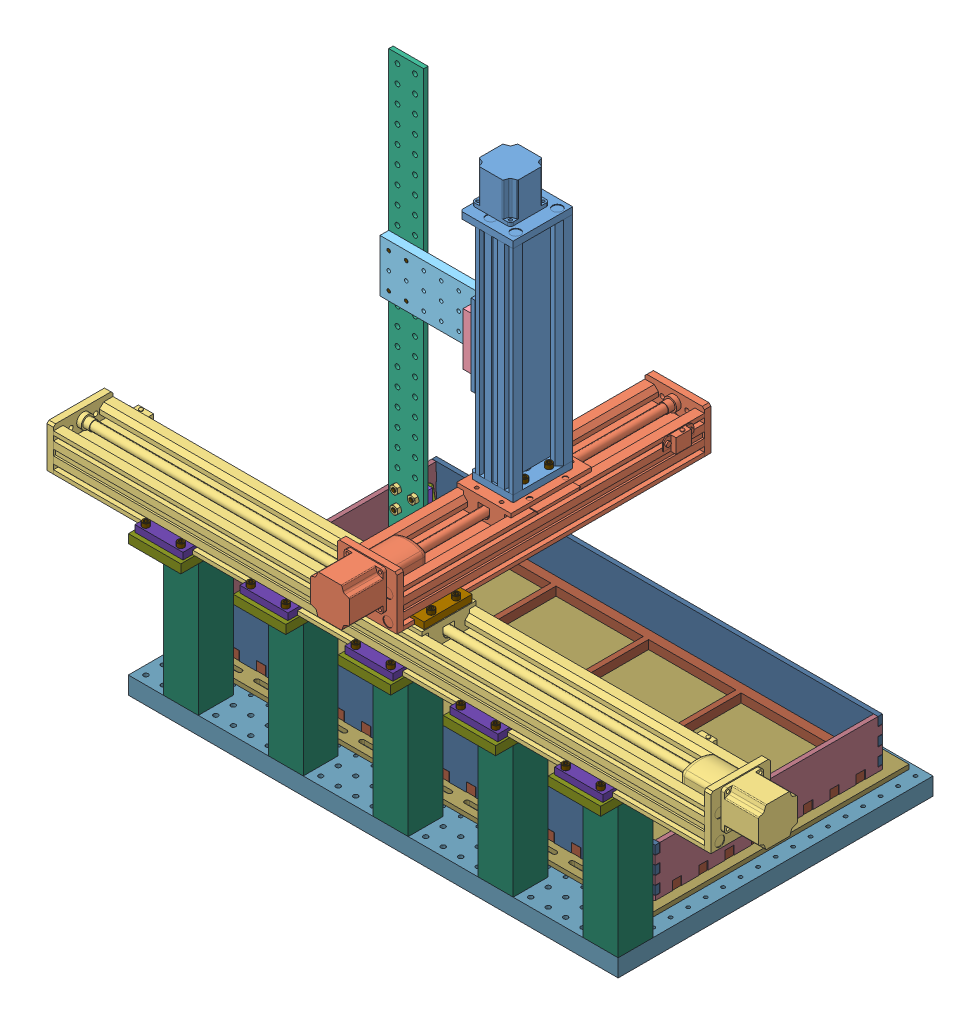
SolidWorks assembly Assem2, configuration Explosion. Lengths in mm.
Overall size (1018.03 802.77 546.22).
126 component instances, 21 part files, 120 mates.
Components (placement in the parent):
- MN10-0050-xxx-21 2Cleats PK266-1: MN10-0050-xxx-21 2Cleats PK266 [Default] at (26.0409 355.727 35.5482) x (0 0 -1) z (0 1 0) size (95.35 76.96 383.03)
- MN10-0100-xxx-21 2Cleats PK266-1: MN10-0100-xxx-21 2Cleats PK266 [Default] at (26.0409 308.3542 -182.8859) size (95.35 76.96 510.03)
- MN10-0300-xxx-21 2Cleats PK266-1: MN10-0300-xxx-21 2Cleats PK266 [Default] at (-446.405 243.2032 203.1941) x (0 0 -1) z (1 0 0) size (95.35 76.96 1018.03)
- Arm-1: Arm [Default] at (-11.8069 510.667 35.5482) x (0 0 1) z (0 -1 0) size (76.2 165.1 609.6)
  - Arm A-1: Arm A [Default] at origin size (76.2 12.7 76.2)
  - Arm B-1: Arm B [Default] at (0 88.9 0) x (0 1 0) z (0 0 1) size (152.4 12.7 76.2)
  - Arm C-1: Arm C [Default] at (-6.35 139.7 38.1) x (0 -1 0) z (0 0 -1) size (50.8 6.35 609.6)
- Verasonics (L11-5v)-1: Verasonics (L11-5v) [Default] at (-151.5069 115.5442 -3.8218) x (-1 0 0) z (0 0 1) size (57.98 122.43 23.49)
- L11_4v_holder_v8-1: L11_4v_holder_v8 [Default] at (-151.5069 155.067 -3.8218) size (50.8 114.3 26.72)
- BiSlide Cleat MC-2-1: BiSlide Cleat MC-2 [Default] at (69.2395 281.051 168.2691) size (20.27 9.74 69.85)
- BiSlide Cleat MC-2-2: BiSlide Cleat MC-2 [Default] at (-17.1695 281.051 238.1191) x (-1 0 0) z (0 0 -1) size (20.27 9.74 69.85)
- Tank-1: Tank [Default] at (-7.3117 0 -28.6003) size (674.12 76.2 382.02)
  - Tank_Long-1: Tank_Long [Default] at (0.508 47.625 -165.1) x (1 0 0) z (0 -1 0) size (647.7 6.35 75.69)
  - Tank_Inner-1: Tank_Inner [Default] at (0 6.35 0) size (647.7 12.7 330.2)
  - Tank_Base-1: Tank_Base [Default] at origin size (674.12 6.35 382.02)
  - Tank_Short-1: Tank_Short [Default] at (-323.342 47.625 0) x (0 0 -1) z (0 -1 0) size (330.2 6.35 75.69)
  - Tank_Short-2: Tank_Short [Default] at (318.008 47.625 -0.254) x (0 0 -1) z (0 -1 0) size (330.2 6.35 75.69)
  - Tank_Long-2: Tank_Long [Default] at (0.508 47.625 158.496) x (1 0 0) z (0 -1 0) size (647.7 6.35 75.69)
- Base-1: Base [Default] x (-1 0 0) z (0 0 -1) size (711.2 25.4 457.2)
- Pillar-5: Pillar [Default] at (330.2 0 203.2) size (50.8 203.2 50.8)
- Mount-1: Mount [Default] at (330.2 203.2 203.2) size (76.2 12.7 127)
- BiSlide Optical Table Cleat MC-3-1: BiSlide Optical Table Cleat MC-3 [Default] at (295.275 215.9 159.9955) x (0 0 -1) z (1 0 0) size (20.27 9.74 69.85)
- BiSlide Optical Table Cleat MC-3-2: BiSlide Optical Table Cleat MC-3 [Default] at (365.125 215.9 246.4045) x (0 0 1) z (-1 0 0) size (20.27 9.74 69.85)
- Screw 0.75-1: Screw 0.75 [92196A540] at (355.6 206.5945 152.4) x (0.967049 0 0.25459) z (0 -1 0) size (9.53 9.53 26.14)
- Screw 0.75-41: Screw 0.75 [92196A540] at (304.8 206.5945 152.4) x (0.928674 0 -0.370897) z (0 -1 0) size (9.53 9.53 26.14)
- Screw 0.75-46: Screw 0.75 [92196A540] at (304.8 206.5945 254) x (0.224681 0 -0.974432) z (0 -1 0) size (9.53 9.53 26.14)
- Screw 0.75-51: Screw 0.75 [92196A540] at (355.6 206.5945 254) x (0.019501 0 -0.99981) z (0 -1 0) size (9.53 9.53 26.14)
- Screw 1.00-2: Screw 1.00 [92196A542] at (317.5 8.89 215.9) x (1 0 0) z (0 1 0) size (9.53 9.53 32.53)
- Screw 1.00-22: Screw 1.00 [92196A542] at (342.9 8.89 215.9) x (1 0 0) z (0 1 0) size (9.53 9.53 32.53)
- Screw 1.00-27: Screw 1.00 [92196A542] at (317.5 8.89 190.5) x (1 0 0) z (0 1 0) size (9.53 9.53 32.53)
- Screw 1.00-32: Screw 1.00 [92196A542] at (342.9 8.89 190.5) x (1 0 0) z (0 1 0) size (9.53 9.53 32.53)
- Screw 0.75-56: Screw 0.75 [92196A540] at (342.9 190.5 215.9) x (0.019501 0 -0.99981) z (0 -1 0) size (9.53 9.53 26.14)
- Screw 0.75-61: Screw 0.75 [92196A540] at (342.9 190.5 190.5) x (0.019501 0 -0.99981) z (0 -1 0) size (9.53 9.53 26.14)
- Screw 0.75-66: Screw 0.75 [92196A540] at (317.5 190.5 215.9) x (0.019501 0 -0.99981) z (0 -1 0) size (9.53 9.53 26.14)
- Screw 0.75-71: Screw 0.75 [92196A540] at (317.5 190.5 190.5) x (0.320717 0 -0.947175) z (0 -1 0) size (9.53 9.53 26.14)
- Screw 0.75-72: Screw 0.75 [92196A540] at (165.1 190.5 190.5) x (0.320717 0 -0.947175) z (0 -1 0) size (9.53 9.53 26.14)
- Screw 0.75-73: Screw 0.75 [92196A540] at (12.7 190.5 190.5) x (0.320717 0 -0.947175) z (0 -1 0) size (9.53 9.53 26.14)
- Screw 0.75-74: Screw 0.75 [92196A540] at (-139.7 190.5 190.5) x (0.320717 0 -0.947175) z (0 -1 0) size (9.53 9.53 26.14)
- Screw 0.75-75: Screw 0.75 [92196A540] at (-292.1 190.5 190.5) x (0.320717 0 -0.947175) z (0 -1 0) size (9.53 9.53 26.14)
- Screw 0.75-67: Screw 0.75 [92196A540] at (165.1 190.5 215.9) x (0.019501 0 -0.99981) z (0 -1 0) size (9.53 9.53 26.14)
- Screw 0.75-68: Screw 0.75 [92196A540] at (12.7 190.5 215.9) x (0.019501 0 -0.99981) z (0 -1 0) size (9.53 9.53 26.14)
- Screw 0.75-69: Screw 0.75 [92196A540] at (-139.7 190.5 215.9) x (0.019501 0 -0.99981) z (0 -1 0) size (9.53 9.53 26.14)
- Screw 0.75-70: Screw 0.75 [92196A540] at (-292.1 190.5 215.9) x (0.019501 0 -0.99981) z (0 -1 0) size (9.53 9.53 26.14)
- Screw 0.75-62: Screw 0.75 [92196A540] at (190.5 190.5 190.5) x (0.019501 0 -0.99981) z (0 -1 0) size (9.53 9.53 26.14)
- Screw 0.75-63: Screw 0.75 [92196A540] at (38.1 190.5 190.5) x (0.019501 0 -0.99981) z (0 -1 0) size (9.53 9.53 26.14)
- Screw 0.75-64: Screw 0.75 [92196A540] at (-114.3 190.5 190.5) x (0.019501 0 -0.99981) z (0 -1 0) size (9.53 9.53 26.14)
- Screw 0.75-65: Screw 0.75 [92196A540] at (-266.7 190.5 190.5) x (0.019501 0 -0.99981) z (0 -1 0) size (9.53 9.53 26.14)
- Screw 0.75-57: Screw 0.75 [92196A540] at (190.5 190.5 215.9) x (0.019501 0 -0.99981) z (0 -1 0) size (9.53 9.53 26.14)
- Screw 0.75-58: Screw 0.75 [92196A540] at (38.1 190.5 215.9) x (0.019501 0 -0.99981) z (0 -1 0) size (9.53 9.53 26.14)
- Screw 0.75-59: Screw 0.75 [92196A540] at (-114.3 190.5 215.9) x (0.019501 0 -0.99981) z (0 -1 0) size (9.53 9.53 26.14)
- Screw 0.75-60: Screw 0.75 [92196A540] at (-266.7 190.5 215.9) x (0.019501 0 -0.99981) z (0 -1 0) size (9.53 9.53 26.14)
- Screw 1.00-33: Screw 1.00 [92196A542] at (190.5 8.89 190.5) x (1 0 0) z (0 1 0) size (9.53 9.53 32.53)
- Screw 1.00-34: Screw 1.00 [92196A542] at (38.1 8.89 190.5) x (1 0 0) z (0 1 0) size (9.53 9.53 32.53)
- Screw 1.00-35: Screw 1.00 [92196A542] at (-114.3 8.89 190.5) x (1 0 0) z (0 1 0) size (9.53 9.53 32.53)
- Screw 1.00-36: Screw 1.00 [92196A542] at (-266.7 8.89 190.5) x (1 0 0) z (0 1 0) size (9.53 9.53 32.53)
- Screw 1.00-28: Screw 1.00 [92196A542] at (165.1 8.89 190.5) x (1 0 0) z (0 1 0) size (9.53 9.53 32.53)
- Screw 1.00-29: Screw 1.00 [92196A542] at (12.7 8.89 190.5) x (1 0 0) z (0 1 0) size (9.53 9.53 32.53)
- Screw 1.00-30: Screw 1.00 [92196A542] at (-139.7 8.89 190.5) x (1 0 0) z (0 1 0) size (9.53 9.53 32.53)
- Screw 1.00-31: Screw 1.00 [92196A542] at (-292.1 8.89 190.5) x (1 0 0) z (0 1 0) size (9.53 9.53 32.53)
- Screw 1.00-23: Screw 1.00 [92196A542] at (190.5 8.89 215.9) x (1 0 0) z (0 1 0) size (9.53 9.53 32.53)
- Screw 1.00-24: Screw 1.00 [92196A542] at (38.1 8.89 215.9) x (1 0 0) z (0 1 0) size (9.53 9.53 32.53)
- Screw 1.00-25: Screw 1.00 [92196A542] at (-114.3 8.89 215.9) x (1 0 0) z (0 1 0) size (9.53 9.53 32.53)
- Screw 1.00-26: Screw 1.00 [92196A542] at (-266.7 8.89 215.9) x (1 0 0) z (0 1 0) size (9.53 9.53 32.53)
- Screw 1.00-18: Screw 1.00 [92196A542] at (165.1 8.89 215.9) x (1 0 0) z (0 1 0) size (9.53 9.53 32.53)
- Screw 1.00-19: Screw 1.00 [92196A542] at (12.7 8.89 215.9) x (1 0 0) z (0 1 0) size (9.53 9.53 32.53)
- Screw 1.00-20: Screw 1.00 [92196A542] at (-139.7 8.89 215.9) x (1 0 0) z (0 1 0) size (9.53 9.53 32.53)
- Screw 1.00-21: Screw 1.00 [92196A542] at (-292.1 8.89 215.9) x (1 0 0) z (0 1 0) size (9.53 9.53 32.53)
- Screw 0.75-52: Screw 0.75 [92196A540] at (203.2 206.5945 254) x (0.019501 0 -0.99981) z (0 -1 0) size (9.53 9.53 26.14)
- Screw 0.75-53: Screw 0.75 [92196A540] at (50.8 206.5945 254) x (0.019501 0 -0.99981) z (0 -1 0) size (9.53 9.53 26.14)
- Screw 0.75-54: Screw 0.75 [92196A540] at (-101.6 206.5945 254) x (0.019501 0 -0.99981) z (0 -1 0) size (9.53 9.53 26.14)
- Screw 0.75-55: Screw 0.75 [92196A540] at (-254 206.5945 254) x (0.019501 0 -0.99981) z (0 -1 0) size (9.53 9.53 26.14)
- Screw 0.75-47: Screw 0.75 [92196A540] at (152.4 206.5945 254) x (0.224681 0 -0.974432) z (0 -1 0) size (9.53 9.53 26.14)
- Screw 0.75-48: Screw 0.75 [92196A540] at (0 206.5945 254) x (0.224681 0 -0.974432) z (0 -1 0) size (9.53 9.53 26.14)
- Screw 0.75-49: Screw 0.75 [92196A540] at (-152.4 206.5945 254) x (0.224681 0 -0.974432) z (0 -1 0) size (9.53 9.53 26.14)
- Screw 0.75-50: Screw 0.75 [92196A540] at (-304.8 206.5945 254) x (0.224681 0 -0.974432) z (0 -1 0) size (9.53 9.53 26.14)
- Screw 0.75-42: Screw 0.75 [92196A540] at (152.4 206.5945 152.4) x (0.928674 0 -0.370897) z (0 -1 0) size (9.53 9.53 26.14)
- Screw 0.75-43: Screw 0.75 [92196A540] at (0 206.5945 152.4) x (0.928674 0 -0.370897) z (0 -1 0) size (9.53 9.53 26.14)
- Screw 0.75-44: Screw 0.75 [92196A540] at (-152.4 206.5945 152.4) x (0.928674 0 -0.370897) z (0 -1 0) size (9.53 9.53 26.14)
- Screw 0.75-45: Screw 0.75 [92196A540] at (-304.8 206.5945 152.4) x (0.928674 0 -0.370897) z (0 -1 0) size (9.53 9.53 26.14)
- Screw 0.75-37: Screw 0.75 [92196A540] at (203.2 206.5945 152.4) x (0.967049 0 0.25459) z (0 -1 0) size (9.53 9.53 26.14)
- Screw 0.75-38: Screw 0.75 [92196A540] at (50.8 206.5945 152.4) x (0.967049 0 0.25459) z (0 -1 0) size (9.53 9.53 26.14)
- Screw 0.75-39: Screw 0.75 [92196A540] at (-101.6 206.5945 152.4) x (0.967049 0 0.25459) z (0 -1 0) size (9.53 9.53 26.14)
- Screw 0.75-40: Screw 0.75 [92196A540] at (-254 206.5945 152.4) x (0.967049 0 0.25459) z (0 -1 0) size (9.53 9.53 26.14)
- BiSlide Optical Table Cleat MC-3-11: BiSlide Optical Table Cleat MC-3 [Default] at (212.725 215.9 246.4045) x (0 0 1) z (-1 0 0) size (20.27 9.74 69.85)
- BiSlide Optical Table Cleat MC-3-12: BiSlide Optical Table Cleat MC-3 [Default] at (60.325 215.9 246.4045) x (0 0 1) z (-1 0 0) size (20.27 9.74 69.85)
- BiSlide Optical Table Cleat MC-3-13: BiSlide Optical Table Cleat MC-3 [Default] at (-92.075 215.9 246.4045) x (0 0 1) z (-1 0 0) size (20.27 9.74 69.85)
- BiSlide Optical Table Cleat MC-3-14: BiSlide Optical Table Cleat MC-3 [Default] at (-244.475 215.9 246.4045) x (0 0 1) z (-1 0 0) size (20.27 9.74 69.85)
- BiSlide Optical Table Cleat MC-3-15: BiSlide Optical Table Cleat MC-3 [Default] at (142.875 215.9 159.9955) x (0 0 -1) z (1 0 0) size (20.27 9.74 69.85)
- BiSlide Optical Table Cleat MC-3-16: BiSlide Optical Table Cleat MC-3 [Default] at (-9.525 215.9 159.9955) x (0 0 -1) z (1 0 0) size (20.27 9.74 69.85)
- BiSlide Optical Table Cleat MC-3-17: BiSlide Optical Table Cleat MC-3 [Default] at (-161.925 215.9 159.9955) x (0 0 -1) z (1 0 0) size (20.27 9.74 69.85)
- BiSlide Optical Table Cleat MC-3-18: BiSlide Optical Table Cleat MC-3 [Default] at (-314.325 215.9 159.9955) x (0 0 -1) z (1 0 0) size (20.27 9.74 69.85)
- Mount-6: Mount [Default] at (177.8 203.2 203.2) size (76.2 12.7 127)
- Mount-7: Mount [Default] at (25.4 203.2 203.2) size (76.2 12.7 127)
- Mount-8: Mount [Default] at (-127 203.2 203.2) size (76.2 12.7 127)
- Mount-9: Mount [Default] at (-279.4 203.2 203.2) size (76.2 12.7 127)
- Pillar-10: Pillar [Default] at (177.8 0 203.2) size (50.8 203.2 50.8)
- Pillar-11: Pillar [Default] at (25.4 0 203.2) size (50.8 203.2 50.8)
- Pillar-12: Pillar [Default] at (-127 0 203.2) size (50.8 203.2 50.8)
- Pillar-13: Pillar [Default] at (-279.4 0 203.2) size (50.8 203.2 50.8)
- Screw 0.75-76: Screw 0.75 [92196A540] at (76.835 271.7455 185.1601) x (0.380553 0 0.924759) z (0 -1 0) size (9.53 9.53 26.14)
- Screw 0.75-77: Screw 0.75 [92196A540] at (76.835 271.7455 221.2281) x (0.931591 0 0.363508) z (0 -1 0) size (9.53 9.53 26.14)
- Screw 0.75-78: Screw 0.75 [92196A540] at (-24.765 271.7455 185.1601) x (-0.20973 0 -0.977759) z (0 -1 0) size (9.53 9.53 26.14)
- Screw 0.75-79: Screw 0.75 [92196A540] at (-24.765 271.7455 221.2281) x (0.199431 0 -0.979912) z (0 -1 0) size (9.53 9.53 26.14)
- Screw 0.75-80: Screw 0.75 [92196A540] at (44.0749 336.677 53.5881) x (0.844393 0 0.535724) z (0 -1 0) size (9.53 9.53 26.14)
- Screw 0.75-81: Screw 0.75 [92196A540] at (44.0749 336.677 17.5201) x (0.224867 0 -0.974389) z (0 -1 0) size (9.53 9.53 26.14)
- Screw 0.75-82: Screw 0.75 [92196A540] at (8.0069 336.677 17.5201) x (-0.995611 0 -0.093586) z (0 -1 0) size (9.53 9.53 26.14)
- Screw 0.75-83: Screw 0.75 [92196A540] at (8.0069 336.677 53.5881) x (-0.995611 0 -0.093586) z (0 -1 0) size (9.53 9.53 26.14)
- Screw 0.50-1: Screw 0.50 [92196A537] at (-5.4569 528.701 53.5822) x (0 0.678478 -0.734621) z (1 0 0) size (9.53 9.53 19.76)
- Screw 0.50-2: Screw 0.50 [92196A537] at (-5.4569 492.633 53.5822) x (0 0.678478 -0.734621) z (1 0 0) size (9.53 9.53 19.76)
- Screw 0.50-4: Screw 0.50 [92196A537] at (-5.4569 492.633 17.5142) x (0 0.678478 -0.734621) z (1 0 0) size (9.53 9.53 19.76)
- Screw 0.50-5: Screw 0.50 [92196A537] at (-5.4569 528.701 17.5142) x (0 0.84628 0.532739) z (1 0 0) size (9.53 9.53 19.76)
- Screw 0.50-6: Screw 0.50 [92196A537] at (-30.8569 485.267 35.5482) x (0 -0.902178 -0.431364) z (-1 0 0) size (9.53 9.53 19.76)
- Screw 0.50-7: Screw 0.50 [92196A537] at (-30.8569 510.667 35.5482) x (0 0.454026 -0.890989) z (-1 0 0) size (9.53 9.53 19.76)
- Screw 0.50-8: Screw 0.50 [92196A537] at (-30.8569 536.067 35.5482) x (0 0.397067 -0.91779) z (-1 0 0) size (9.53 9.53 19.76)
- Screw 0.75-84: Screw 0.75 [92196A540] at (-138.8069 536.067 41.8982) x (0.718354 -0.695678 0) z (0 0 1) size (9.53 9.53 26.14)
- Screw 0.75-85: Screw 0.75 [92196A540] at (-164.2069 536.067 41.8982) x (-0.621869 -0.783122 0) z (0 0 1) size (9.53 9.53 26.14)
- Screw 0.75-86: Screw 0.75 [92196A540] at (-138.8069 485.267 41.8982) x (-0.621869 -0.783122 0) z (0 0 1) size (9.53 9.53 26.14)
- Screw 0.75-87: Screw 0.75 [92196A540] at (-164.2069 485.267 41.8982) x (-0.621869 -0.783122 0) z (0 0 1) size (9.53 9.53 26.14)
- Screw 0.75-88: Screw 0.75 [92196A540] at (-164.2069 205.867 35.5482) x (-0.621869 -0.783122 0) z (0 0 1) size (9.53 9.53 26.14)
- Screw 0.75-89: Screw 0.75 [92196A540] at (-138.8069 231.267 35.5482) x (-0.621869 -0.783122 0) z (0 0 1) size (9.53 9.53 26.14)
- Screw 0.75-90: Screw 0.75 [92196A540] at (-138.8069 205.867 35.5482) x (-0.621869 -0.783122 0) z (0 0 1) size (9.53 9.53 26.14)
- Screw 0.75-91: Screw 0.75 [92196A540] at (-164.2069 231.267 35.5482) x (-0.621869 -0.783122 0) z (0 0 1) size (9.53 9.53 26.14)
- Nut-1: Nut [91845A029] at (-164.2069 231.267 31.9763) x (0.978932 0.204188 0) z (0 0 1) size (11.11 12.83 6.51)
- Nut-2: Nut [91845A029] at (-138.8069 231.267 31.9763) x (0.978932 0.204188 0) z (0 0 1) size (11.11 12.83 6.51)
- Nut-3: Nut [91845A029] at (-164.2069 205.867 31.9763) x (0.978932 0.204188 0) z (0 0 1) size (11.11 12.83 6.51)
- Nut-4: Nut [91845A029] at (-138.8069 205.867 31.9763) x (0.978932 0.204188 0) z (0 0 1) size (11.11 12.83 6.51)
Mates (geometry in assembly coordinates):
- Coincident64: coincident anti-aligned: plane of MN10-0300-xxx-21 2Cleats PK266-1 through (-446.405 221.6132 159.9946) normal (0 0 -1); plane of BiSlide Optical Table Cleat MC-3-1 through (295.275 218.7566 159.9946) normal (0 0 1)
- Coincident65: coincident anti-aligned: plane of MN10-0300-xxx-21 2Cleats PK266-1 through (-446.405 221.6132 166.7583) normal (0 1 0); plane of BiSlide Optical Table Cleat MC-3-1 through (295.275 221.6132 163.1569) normal (0 -1 0)
- Coincident66: coincident anti-aligned: plane of Pillar-5 through (330.2 203.2 203.2) normal (0 1 0); plane of Mount-1 through (330.2 203.2 203.2) normal (0 -1 0)
- Parallel1: parallel aligned: plane of Pillar-5 through (304.8 203.2 177.8) normal (0 0 -1); plane of Mount-1 through (292.1 215.9 139.7) normal (0 0 -1)
- Coincident67: coincident anti-aligned: plane of MN10-0300-xxx-21 2Cleats PK266-1 through (-446.405 215.9 246.4054) normal (0 0 1); plane of BiSlide Optical Table Cleat MC-3-2 through (365.125 218.7566 246.4054) normal (0 0 -1)
- Coincident68: coincident anti-aligned: plane of MN10-0300-xxx-21 2Cleats PK266-1 through (-446.405 221.6132 246.4054) normal (0 1 0); plane of BiSlide Optical Table Cleat MC-3-2 through (365.125 221.6132 243.2431) normal (0 -1 0)
- Coincident69: coincident anti-aligned: plane of MN10-0300-xxx-21 2Cleats PK266-1 through (-446.405 215.9 232.7392) normal (0 -1 0); plane of Mount-1 through (330.2 215.9 203.2) normal (0 1 0)
- Coincident70: coincident anti-aligned: plane of MN10-0300-xxx-21 2Cleats PK266-1 through (-32.385 281.051 242.5439) normal (0 1 0); plane of MN10-0100-xxx-21 2Cleats PK266-1 through (69.2404 281.051 253.9941) normal (0 -1 0)
- Parallel2: parallel anti-aligned: line of MN10-0300-xxx-21 2Cleats PK266-1 through (84.455 275.3631 242.5439) axis (0 1 0); line of MN10-0100-xxx-21 2Cleats PK266-1 through (69.2404 355.0614 263.5191) axis (0 -1 0)
- Coincident74: coincident anti-aligned: plane of MN10-0100-xxx-21 2Cleats PK266-1 through (-13.3089 346.202 -22.8659) normal (0 1 0); plane of MN10-0050-xxx-21 2Cleats PK266-1 through (22.7334 346.202 35.5546) normal (0 -1 0)
- Parallel3: parallel aligned: plane of MN10-0100-xxx-21 2Cleats PK266-1 through (26.0347 328.2952 317.6211) normal (0 0 1); plane of MN10-0050-xxx-21 2Cleats PK266-1 through (21.8502 355.727 78.7595) normal (0 0 1)
- Coincident75: coincident anti-aligned: plane of Base-1 through (0 0 0) normal (0 1 0); plane of Tank-1/Tank_Base-1 through (-7.3117 0 -28.6003) normal (0 -1 0)
- Concentric35: concentric anti-aligned: circle of L11_4v_holder_v8-1; circle of Verasonics (L11-5v)-1
- Parallel8: parallel aligned: plane of L11_4v_holder_v8-1 through (-176.9069 104.267 10.1482) normal (-1 0 0); plane of Verasonics (L11-5v)-1 through (-151.5069 115.5442 -3.8218) normal (-1 0 0)
- Distance2: distance = 44.0772 mm aligned: plane of Verasonics (L11-5v)-1 through (-151.5069 224.5442 -3.8218) normal (0 1 0); plane of L11_4v_holder_v8-1 through (-151.5069 180.467 -3.8218) normal (0 1 0)
- Parallel9: parallel aligned: plane of MN10-0050-xxx-21 2Cleats PK266-1 through (1.2787 569.087 35.5482) normal (0 1 0); plane of Arm-1/Arm B-1 through (-24.5069 548.767 29.1982) normal (0 1 0)
- Parallel10: parallel aligned: plane of Arm-1/Arm C-1 through (-176.9069 777.367 22.8482) normal (-1 0 0); plane of L11_4v_holder_v8-1 through (-176.9069 104.267 10.1482) normal (-1 0 0)
- Concentric38: concentric aligned: circle of Arm-1/Arm C-1; circle of L11_4v_holder_v8-1
- Concentric39: concentric aligned: circle of Arm-1/Arm C-1; circle of L11_4v_holder_v8-1
- Coincident81: coincident anti-aligned: plane of Arm-1/Arm C-1 through (-151.5069 472.567 22.8482) normal (0 0 -1); plane of L11_4v_holder_v8-1 through (-151.5069 155.067 22.8482) normal (0 0 1)
- Coincident82: coincident anti-aligned: plane of MN10-0050-xxx-21 2Cleats PK266-1 through (-11.8069 452.247 74.898) normal (-1 0 0); plane of Arm-1/Arm A-1 through (-11.8069 510.667 35.5482) normal (1 0 0)
- Concentric41: concentric anti-aligned: circle of MN10-0050-xxx-21 2Cleats PK266-1; circle of Arm-1/Arm A-1
- Coincident83: coincident anti-aligned: plane of MN10-0300-xxx-21 2Cleats PK266-1 through (-32.385 281.051 242.5439) normal (0 1 0); plane of BiSlide Cleat MC-2-1 through (83.185 281.051 168.2691) normal (0 -1 0)
- Concentric42: concentric aligned: circle of MN10-0300-xxx-21 2Cleats PK266-1; circle of BiSlide Cleat MC-2-1
- Parallel11: parallel aligned: plane of MN10-0300-xxx-21 2Cleats PK266-1 through (84.455 267.9653 203.1941) normal (1 0 0); plane of BiSlide Cleat MC-2-1 through (83.185 290.7955 168.2691) normal (1 0 0)
- Distance3: distance = 25.4 mm aligned: plane of MN10-0100-xxx-21 2Cleats PK266-1 through (26.0345 319.1099 263.5191) normal (0 0 1); plane of BiSlide Cleat MC-2-1 through (73.6524 286.5252 238.1191) normal (0 0 1)
- Concentric43: concentric anti-aligned: circle of MN10-0300-xxx-21 2Cleats PK266-1; cylinder of BiSlide Cleat MC-2-2 through (-24.765 217.4142 185.1601) axis (0 1 0) radius 3.4544
- Parallel12: parallel aligned: plane of MN10-0300-xxx-21 2Cleats PK266-1 through (-32.385 267.9653 203.1941) normal (-1 0 0); plane of BiSlide Cleat MC-2-2 through (-31.115 290.7955 238.1191) normal (-1 0 0)
- Coincident84: coincident anti-aligned: plane of MN10-0300-xxx-21 2Cleats PK266-1 through (-32.385 281.051 242.5439) normal (0 1 0); plane of BiSlide Cleat MC-2-2 through (-31.115 281.051 238.1191) normal (0 -1 0)
- Concentric47: concentric aligned: circle of BiSlide Optical Table Cleat MC-3-1; cylinder of Screw 0.75-1 through (355.6 231.9945 152.4) axis (0 -1 0) radius 4.7625
- Concentric48: concentric aligned: cylinder of BiSlide Optical Table Cleat MC-3-1 through (355.6 152.2632 152.4) axis (0 1 0) radius 3.4544; cylinder of Mount-1 through (355.6 215.9 152.4) axis (0 1 0) radius 2.5527
- Coincident87: coincident anti-aligned: plane of BiSlide Optical Table Cleat MC-3-1 through (295.275 225.6445 156.1846) normal (0 1 0); plane of Screw 0.75-1 through (355.6 225.6445 152.4) normal (0 -1 0)
- Coincident88: coincident anti-aligned: plane of BiSlide Optical Table Cleat MC-3-1 through (295.275 225.6445 156.1846) normal (0 1 0); plane of Screw 0.75-41 through (304.8 225.6445 152.4) normal (0 -1 0)
- Concentric49: concentric anti-aligned: cylinder of BiSlide Optical Table Cleat MC-3-1 through (304.8 152.2632 152.4) axis (0 1 0) radius 3.4544; cylinder of Screw 0.75-41 through (304.8 231.9945 152.4) axis (0 -1 0) radius 4.7625
- Concentric50: concentric aligned: cylinder of BiSlide Optical Table Cleat MC-3-2 through (304.8 152.2632 254) axis (0 1 0) radius 3.4544; cylinder of Mount-1 through (304.8 215.9 254) axis (0 1 0) radius 2.5527
- Concentric51: concentric anti-aligned: cylinder of BiSlide Optical Table Cleat MC-3-2 through (355.6 152.2632 254) axis (0 1 0) radius 3.4544; cylinder of Screw 0.75-51 through (355.6 231.9945 254) axis (0 -1 0) radius 4.7625
- Concentric52: concentric anti-aligned: cylinder of BiSlide Optical Table Cleat MC-3-2 through (304.8 152.2632 254) axis (0 1 0) radius 3.4544; cylinder of Screw 0.75-46 through (304.8 231.9945 254) axis (0 -1 0) radius 4.7625
- Coincident89: coincident aligned: plane of Screw 0.75-1 through (355.6 231.9945 152.4) normal (0 1 0); plane of Screw 0.75-51 through (355.6 231.9945 254) normal (0 1 0)
- Coincident90: coincident aligned: plane of Screw 0.75-46 through (304.8 231.9945 254) normal (0 1 0); plane of Screw 0.75-51 through (355.6 231.9945 254) normal (0 1 0)
- Coincident91: coincident aligned: plane of Base-1 through (0 0 0) normal (0 1 0); plane of assembly through (0 0 0) normal (0 1 0)
- Coincident92: coincident anti-aligned: plane of Base-1 through (0 0 0) normal (-1 0 0); plane of assembly through (0 0 0) normal (1 0 0)
- Coincident93: coincident anti-aligned: plane of Base-1 through (0 0 0) normal (0 0 -1); plane of assembly through (0 0 0) normal (0 0 1)
- Coincident94: coincident anti-aligned: plane of Base-1 through (288.7218 -16.51 215.9) normal (0 -1 0); plane of Screw 1.00-2 through (317.5 -16.51 215.9) normal (0 1 0)
- Concentric54: concentric anti-aligned: cylinder of Base-1 through (317.5 -25.4 215.9) axis (0 -1 0) radius 5.5563; cylinder of Screw 1.00-2 through (317.5 -22.86 215.9) axis (0 1 0) radius 4.7625
- Concentric56: concentric anti-aligned: cylinder of Base-1 through (342.9 -25.4 215.9) axis (0 -1 0) radius 5.5563; cylinder of Screw 1.00-22 through (342.9 -22.86 215.9) axis (0 1 0) radius 4.7625
- Concentric57: concentric anti-aligned: cylinder of Base-1 through (317.5 -25.4 190.5) axis (0 -1 0) radius 5.5563; cylinder of Screw 1.00-27 through (317.5 -22.86 190.5) axis (0 1 0) radius 4.7625
- Concentric58: concentric anti-aligned: cylinder of Base-1 through (342.9 -25.4 190.5) axis (0 -1 0) radius 5.5563; cylinder of Screw 1.00-32 through (342.9 -22.86 190.5) axis (0 1 0) radius 4.7625
- Coincident96: coincident aligned: plane of Screw 1.00-2 through (319.8813 -19.2881 211.7756) normal (0 -1 0); plane of Screw 1.00-32 through (345.2812 -19.2881 186.3756) normal (0 -1 0)
- Coincident97: coincident aligned: plane of Screw 1.00-22 through (345.2812 -19.2881 211.7756) normal (0 -1 0); plane of Screw 1.00-32 through (345.2812 -19.2881 186.3756) normal (0 -1 0)
- Coincident98: coincident aligned: plane of Screw 1.00-27 through (319.8813 -19.2881 186.3756) normal (0 -1 0); plane of Screw 1.00-32 through (345.2812 -19.2881 186.3756) normal (0 -1 0)
- Coincident99: coincident anti-aligned: plane of Pillar-5 through (330.2 0 203.2) normal (0 -1 0); plane of Base-1 through (0 0 0) normal (0 1 0)
- Concentric61: concentric anti-aligned: cylinder of Mount-1 through (342.9 215.9 215.9) axis (0 1 0) radius 5.5563; cylinder of Screw 0.75-56 through (342.9 215.9 215.9) axis (0 -1 0) radius 4.7625
- Concentric62: concentric anti-aligned: cylinder of Mount-1 through (317.5 215.9 215.9) axis (0 1 0) radius 5.5563; cylinder of Screw 0.75-66 through (317.5 215.9 215.9) axis (0 -1 0) radius 4.7625
- Concentric63: concentric anti-aligned: cylinder of Mount-1 through (342.9 215.9 190.5) axis (0 1 0) radius 5.5563; cylinder of Screw 0.75-61 through (342.9 215.9 190.5) axis (0 -1 0) radius 4.7625
- Concentric64: concentric anti-aligned: cylinder of Mount-1 through (317.5 215.9 190.5) axis (0 1 0) radius 5.5563; cylinder of Screw 0.75-71 through (317.5 215.9 190.5) axis (0 -1 0) radius 4.7625
- Parallel13: parallel aligned: plane of Pillar-5 through (355.6 203.2 228.6) normal (1 0 0); plane of Base-1 through (355.6 -25.4 -228.6) normal (1 0 0)
- Coincident100: coincident anti-aligned: plane of Mount-1 through (320.8782 209.55 190.5) normal (0 1 0); plane of Screw 0.75-71 through (317.5 209.55 190.5) normal (0 -1 0)
- Coincident101: coincident aligned: plane of Screw 0.75-61 through (347.0701 212.3281 188.1996) normal (0 1 0); plane of Screw 0.75-71 through (322.1703 212.3281 189.5673) normal (0 1 0)
- Coincident102: coincident aligned: plane of Screw 0.75-56 through (347.0701 212.3281 213.5996) normal (0 1 0); plane of Screw 0.75-61 through (347.0701 212.3281 188.1996) normal (0 1 0)
- Coincident103: coincident aligned: plane of Screw 0.75-56 through (347.0701 212.3281 213.5996) normal (0 1 0); plane of Screw 0.75-66 through (321.6701 212.3281 213.5996) normal (0 1 0)
- Coincident104: coincident aligned: plane of Pillar-5 through (304.8 203.2 228.6) normal (0 0 1); plane of Base-1 through (355.6 -25.4 228.6) normal (0 0 1)
- Coincident105: coincident aligned: plane of Pillar-5 through (355.6 203.2 228.6) normal (1 0 0); plane of Base-1 through (355.6 -25.4 -228.6) normal (1 0 0)
- Concentric65: concentric aligned: circle of Mount-1; circle of Pillar-5
- Distance4: distance = 152.4 mm aligned: plane of MN10-0300-xxx-21 2Cleats PK266-1 through (508 253.9589 203.2005) normal (1 0 0); plane of Pillar-5 through (355.6 203.2 228.6) normal (1 0 0)
- Coincident106: coincident anti-aligned: plane of MN10-0100-xxx-21 2Cleats PK266-1 through (69.2404 286.7642 -182.8859) normal (1 0 0); plane of BiSlide Cleat MC-2-1 through (69.2404 281.051 168.2691) normal (-1 0 0)
- Concentric66: concentric aligned: circle of BiSlide Cleat MC-2-1; cylinder of Screw 0.75-77 through (76.835 297.1455 221.2281) axis (0 -1 0) radius 4.7625
- Concentric67: concentric aligned: circle of BiSlide Cleat MC-2-1; cylinder of Screw 0.75-76 through (76.835 297.1455 185.1601) axis (0 -1 0) radius 4.7625
- Concentric68: concentric aligned: circle of BiSlide Cleat MC-2-2; circle of Screw 0.75-79
- Concentric69: concentric aligned: circle of BiSlide Cleat MC-2-2; circle of Screw 0.75-78
- Coincident107: coincident anti-aligned: plane of BiSlide Cleat MC-2-2 through (-10.8458 290.7955 238.1191) normal (0 1 0); plane of Screw 0.75-78 through (-24.765 290.7955 185.1601) normal (0 -1 0)
- Coincident108: coincident aligned: plane of Screw 0.75-78 through (-21.2317 293.5736 181.9668) normal (0 1 0); plane of Screw 0.75-79 through (-20.2485 293.5736 219.7172) normal (0 1 0)
- Coincident109: coincident aligned: plane of Screw 0.75-77 through (77.5541 293.5736 225.936) normal (0 1 0); plane of Screw 0.75-79 through (-20.2485 293.5736 219.7172) normal (0 1 0)
- Coincident110: coincident aligned: plane of Screw 0.75-76 through (73.9271 293.5736 188.9317) normal (0 1 0); plane of Screw 0.75-77 through (77.5541 293.5736 225.936) normal (0 1 0)
- Concentric70: concentric aligned: circle of MN10-0050-xxx-21 2Cleats PK266-1; circle of MN10-0100-xxx-21 2Cleats PK266-1
- Concentric71: concentric anti-aligned: cylinder of MN10-0050-xxx-21 2Cleats PK266-1 through (44.0749 239.4379 53.5881) axis (0 1 0) radius 3.2639; cylinder of Screw 0.75-80 through (44.0749 362.077 53.5881) axis (0 -1 0) radius 4.7625
- Concentric72: concentric anti-aligned: cylinder of MN10-0050-xxx-21 2Cleats PK266-1 through (44.0749 239.4379 17.5201) axis (0 1 0) radius 3.2639; cylinder of Screw 0.75-81 through (44.0749 362.077 17.5201) axis (0 -1 0) radius 4.7625
- Concentric73: concentric aligned: circle of MN10-0050-xxx-21 2Cleats PK266-1; cylinder of Screw 0.75-82 through (8.0069 362.077 17.5201) axis (0 -1 0) radius 4.7625
- Concentric74: concentric anti-aligned: cylinder of MN10-0050-xxx-21 2Cleats PK266-1 through (8.0069 239.4379 53.5881) axis (0 1 0) radius 3.2639; cylinder of Screw 0.75-83 through (8.0069 362.077 53.5881) axis (0 -1 0) radius 4.7625
- Coincident111: coincident anti-aligned: plane of MN10-0050-xxx-21 2Cleats PK266-1 through (22.7334 355.727 35.5546) normal (0 1 0); plane of Screw 0.75-83 through (8.0069 355.727 53.5881) normal (0 -1 0)
- Coincident112: coincident aligned: plane of Screw 0.75-82 through (8.0069 362.077 17.5201) normal (0 1 0); plane of Screw 0.75-83 through (8.0069 362.077 53.5881) normal (0 1 0)
- Coincident113: coincident aligned: plane of Screw 0.75-80 through (44.0749 362.077 53.5881) normal (0 1 0); plane of Screw 0.75-83 through (8.0069 362.077 53.5881) normal (0 1 0)
- Coincident114: coincident aligned: plane of Screw 0.75-81 through (44.0749 362.077 17.5201) normal (0 1 0); plane of Screw 0.75-83 through (8.0069 362.077 53.5881) normal (0 1 0)
- Concentric75: concentric anti-aligned: cylinder of Arm-1/Arm A-1 through (-24.5069 528.701 53.5822) axis (-1 0 0) radius 5.5563; cylinder of Screw 0.50-1 through (-24.5069 528.701 53.5822) axis (1 0 0) radius 4.7625
- Concentric76: concentric anti-aligned: cylinder of Arm-1/Arm A-1 through (-24.5069 528.701 17.5142) axis (-1 0 0) radius 5.5563; cylinder of Screw 0.50-5 through (-24.5069 528.701 17.5142) axis (1 0 0) radius 4.7625
- Concentric77: concentric anti-aligned: cylinder of Arm-1/Arm A-1 through (-24.5069 492.633 17.5142) axis (-1 0 0) radius 5.5563; cylinder of Screw 0.50-4 through (-24.5069 492.633 17.5142) axis (1 0 0) radius 4.7625
- Coincident117: coincident anti-aligned: plane of Arm-1/Arm A-1 through (-18.1569 492.633 20.8924) normal (-1 0 0); plane of Screw 0.50-4 through (-18.1569 492.633 17.5142) normal (1 0 0)
- Coincident118: coincident aligned: plane of Screw 0.50-4 through (-20.9351 497.2785 18.5632) normal (-1 0 0); plane of Screw 0.50-5 through (-20.9351 528.519 22.2732) normal (-1 0 0)
- Coincident119: coincident aligned: plane of Screw 0.50-1 through (-20.9351 533.3465 54.6312) normal (-1 0 0); plane of Screw 0.50-5 through (-20.9351 528.519 22.2732) normal (-1 0 0)
- Coincident120: coincident aligned: plane of Screw 0.50-1 through (-20.9351 533.3465 54.6312) normal (-1 0 0); plane of Screw 0.50-2 through (-20.9351 497.2785 54.6312) normal (-1 0 0)
- Concentric78: concentric anti-aligned: cylinder of Arm-1/Arm A-1 through (-24.5069 492.633 53.5822) axis (-1 0 0) radius 5.5563; cylinder of Screw 0.50-2 through (-24.5069 492.633 53.5822) axis (1 0 0) radius 4.7625
- Concentric79: concentric anti-aligned: cylinder of Arm-1/Arm A-1 through (-11.8069 536.067 35.5482) axis (1 0 0) radius 5.5563; cylinder of Screw 0.50-8 through (-11.8069 536.067 35.5482) axis (-1 0 0) radius 4.7625
- Concentric80: concentric anti-aligned: cylinder of Arm-1/Arm A-1 through (-11.8069 510.667 35.5482) axis (1 0 0) radius 5.5563; cylinder of Screw 0.50-7 through (-11.8069 510.667 35.5482) axis (-1 0 0) radius 4.7625
- Concentric81: concentric anti-aligned: cylinder of Arm-1/Arm A-1 through (-11.8069 485.267 35.5482) axis (1 0 0) radius 5.5563; cylinder of Screw 0.50-6 through (-11.8069 485.267 35.5482) axis (-1 0 0) radius 4.7625
- Coincident121: coincident anti-aligned: plane of Arm-1/Arm A-1 through (-18.1569 536.067 38.9264) normal (1 0 0); plane of Screw 0.50-8 through (-18.1569 536.067 35.5482) normal (-1 0 0)
- Coincident122: coincident anti-aligned: plane of Arm-1/Arm A-1 through (-18.1569 510.667 38.9264) normal (1 0 0); plane of Screw 0.50-7 through (-18.1569 510.667 35.5482) normal (-1 0 0)
- Coincident123: coincident anti-aligned: plane of Arm-1/Arm A-1 through (-18.1569 485.267 38.9264) normal (1 0 0); plane of Screw 0.50-6 through (-18.1569 485.267 35.5482) normal (-1 0 0)
- Concentric86: concentric anti-aligned: circle of Arm-1/Arm B-1; cylinder of Screw 0.75-84 through (-138.8069 536.067 16.4982) axis (0 0 1) radius 4.7625
- Concentric87: concentric aligned: cylinder of Arm-1/Arm C-1 through (-164.2069 536.067 22.8482) axis (0 0 1) radius 3.429; cylinder of Screw 0.75-85 through (-164.2069 536.067 16.4982) axis (0 0 1) radius 4.7625
- Concentric88: concentric aligned: cylinder of Arm-1/Arm C-1 through (-138.8069 485.267 22.8482) axis (0 0 1) radius 3.429; cylinder of Screw 0.75-86 through (-138.8069 485.267 16.4982) axis (0 0 1) radius 4.7625
- Concentric89: concentric aligned: cylinder of Arm-1/Arm C-1 through (-164.2069 485.267 22.8482) axis (0 0 1) radius 3.429; cylinder of Screw 0.75-87 through (-164.2069 485.267 16.4982) axis (0 0 1) radius 4.7625
- Coincident129: coincident anti-aligned: plane of Arm-1/Arm C-1 through (-151.5069 472.567 22.8482) normal (0 0 -1); plane of Screw 0.75-84 through (-138.8069 536.067 22.8482) normal (0 0 1)
- Coincident130: coincident aligned: plane of Screw 0.75-84 through (-134.2271 537.3732 20.0701) normal (0 0 -1); plane of Screw 0.75-85 through (-162.4578 531.6373 20.0701) normal (0 0 -1)
- Coincident131: coincident aligned: plane of Screw 0.75-85 through (-162.4578 531.6373 20.0701) normal (0 0 -1); plane of Screw 0.75-87 through (-162.4578 480.8373 20.0701) normal (0 0 -1)
- Coincident132: coincident aligned: plane of Screw 0.75-86 through (-137.0578 480.8373 20.0701) normal (0 0 -1); plane of Screw 0.75-87 through (-162.4578 480.8373 20.0701) normal (0 0 -1)
- Concentric90: concentric anti-aligned: circle of L11_4v_holder_v8-1; cylinder of Screw 0.75-91 through (-164.2069 231.267 10.1482) axis (0 0 1) radius 4.7625
- Concentric91: concentric anti-aligned: circle of L11_4v_holder_v8-1; cylinder of Screw 0.75-88 through (-164.2069 205.867 10.1482) axis (0 0 1) radius 4.7625
- Concentric92: concentric anti-aligned: cylinder of L11_4v_holder_v8-1 through (-138.8069 231.267 22.8482) axis (0 0 -1) radius 3.429; cylinder of Screw 0.75-89 through (-138.8069 231.267 10.1482) axis (0 0 1) radius 4.7625
- Concentric93: concentric anti-aligned: cylinder of L11_4v_holder_v8-1 through (-138.8069 205.867 22.8482) axis (0 0 -1) radius 3.429; cylinder of Screw 0.75-90 through (-138.8069 205.867 10.1482) axis (0 0 1) radius 4.7625
- Coincident133: coincident anti-aligned: plane of L11_4v_holder_v8-1 through (-151.5069 155.067 16.4982) normal (0 0 -1); plane of Screw 0.75-88 through (-164.2069 205.867 16.4982) normal (0 0 1)
- Coincident134: coincident aligned: plane of Screw 0.75-88 through (-162.4578 201.4373 13.7201) normal (0 0 -1); plane of Screw 0.75-91 through (-162.4578 226.8373 13.7201) normal (0 0 -1)
- Coincident135: coincident aligned: plane of Screw 0.75-89 through (-137.0578 226.8373 13.7201) normal (0 0 -1); plane of Screw 0.75-91 through (-162.4578 226.8373 13.7201) normal (0 0 -1)
- Coincident136: coincident aligned: plane of Screw 0.75-89 through (-137.0578 226.8373 13.7201) normal (0 0 -1); plane of Screw 0.75-90 through (-137.0578 201.4373 13.7201) normal (0 0 -1)
- Concentric94: concentric anti-aligned: cylinder of Screw 0.75-91 through (-164.2069 231.267 10.1482) axis (0 0 1) radius 4.7625; circle of Nut-1
- Coincident137: coincident anti-aligned: plane of Arm-1/Arm C-1 through (-151.5069 472.567 29.1982) normal (0 0 1); plane of Nut-1 through (-170.3011 233.2728 29.1982) normal (0 0 -1)
- Concentric95: concentric anti-aligned: circle of Arm-1/Arm C-1; circle of Nut-2
- Concentric96: concentric anti-aligned: circle of Arm-1/Arm C-1; circle of Nut-3
- Concentric97: concentric anti-aligned: circle of Arm-1/Arm C-1; circle of Nut-4
- Coincident138: coincident aligned: plane of Nut-3 through (-164.2069 205.867 31.9763) normal (0 0 1); plane of Nut-4 through (-138.8069 205.867 31.9763) normal (0 0 1)
- Coincident139: coincident aligned: plane of Nut-2 through (-138.8069 231.267 31.9763) normal (0 0 1); plane of Nut-3 through (-164.2069 205.867 31.9763) normal (0 0 1)
- Coincident140: coincident aligned: plane of Nut-1 through (-164.2069 231.267 31.9763) normal (0 0 1); plane of Nut-2 through (-138.8069 231.267 31.9763) normal (0 0 1)
